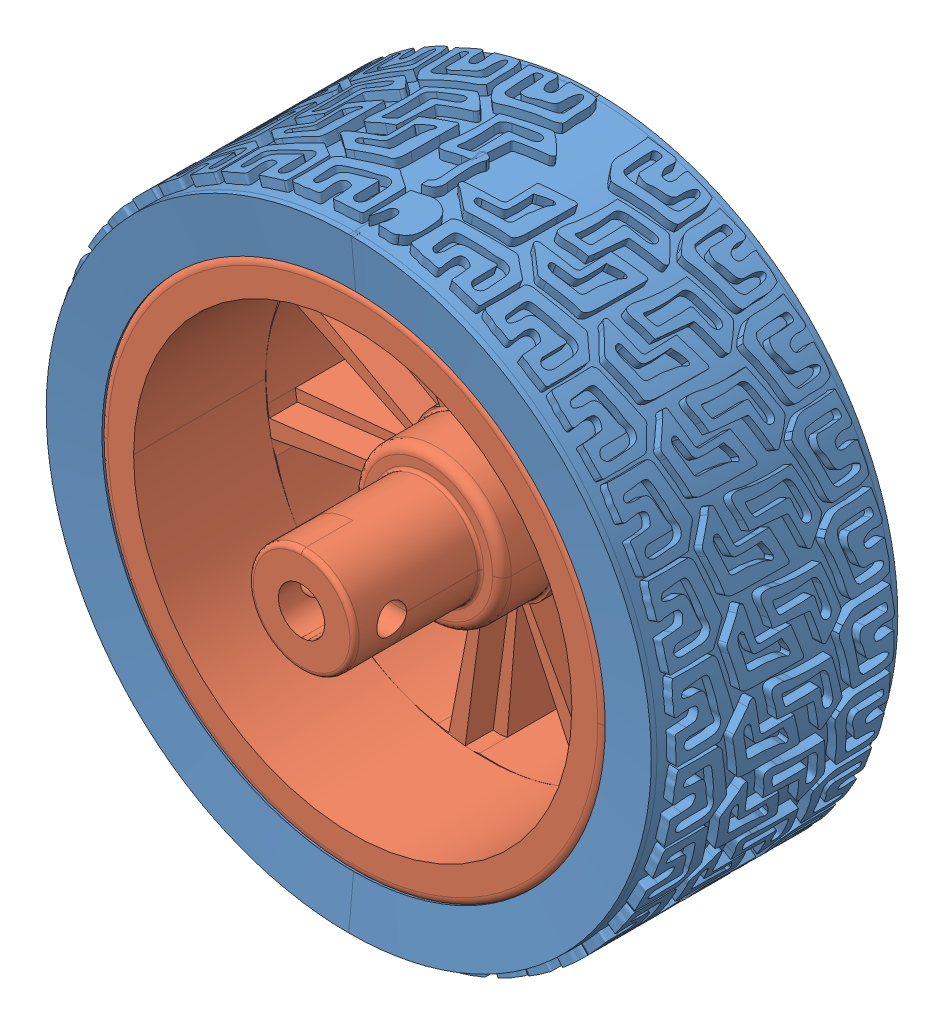
SolidWorks assembly 蓝色橡胶轮胎, configuration 默认. Lengths in mm.
Overall size (67.13 67.1 31.57).
3 component instances, 2 part files, 0 mates.
Components (placement in the parent):
- 蓝色橡胶轮胎.stp-1: 蓝色橡胶轮胎.stp [默认] at origin size (67.13 67.1 31.57)
  - PRT0002.stp-1: PRT0002.stp [默认] at (33.8013 60.8485 -25.75) size (67.13 67.1 26.5)
  - LUNGU2.stp-1: LUNGU2.stp [默认] at (61.1013 33.7786 -26.4276) x (0 0 1) z (-1 0.000833 0) size (31.5 54.6 54.6)
